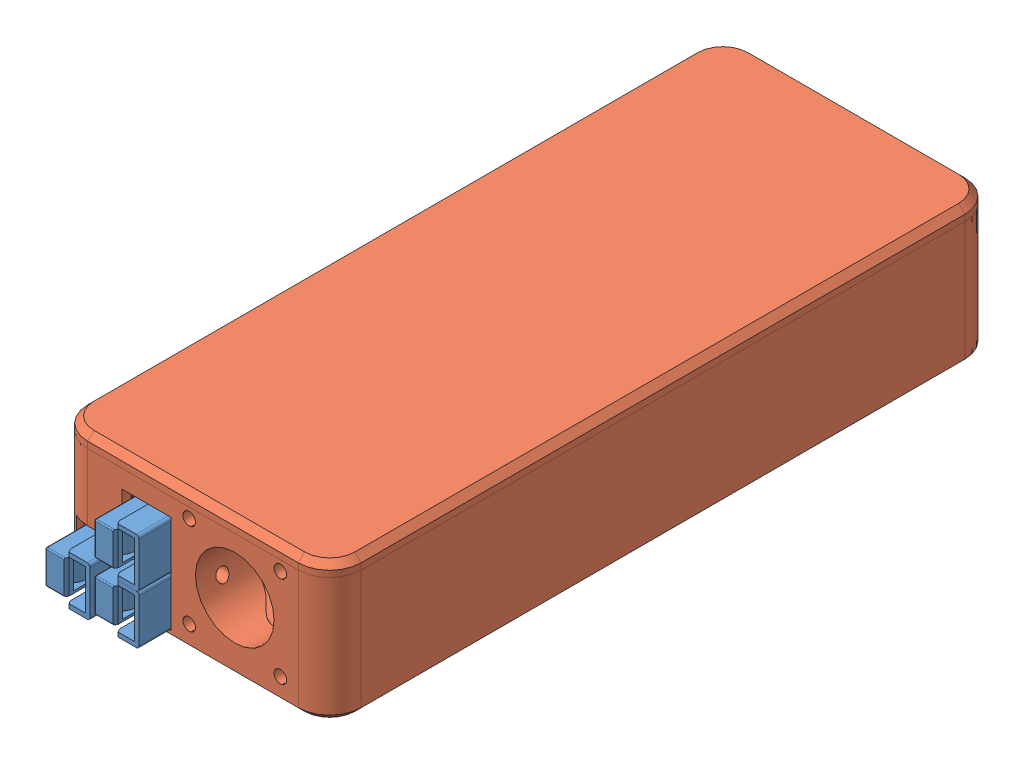
SolidWorks assembly AxxSolder_Portable, configuration Default. Lengths in mm.
Overall size (43.5 41.05 111.1).
6 component instances, 3 part files, 9 mates.
Components (placement in the parent):
- Anderson_PowerPole-3: Anderson_PowerPole [Default] at (-7.3715 3.9141 34.4539) x (0 -1 0) z (0 0 1) size (16.24 16.24 22.71)
  - powerpole 15-45A housing.step-3: powerpole 15-45A housing.step [Default] at origin size (8.44 8.44 22.71)
  - powerpole 15-45A housing.step-5: powerpole 15-45A housing.step [Default] at (-7.8 0 0) size (8.44 8.44 22.71)
  - powerpole 15-45A housing.step-6: powerpole 15-45A housing.step [Default] at (0 -7.8 0) size (8.44 8.44 22.71)
- Encolsure_Portable-1: Encolsure_Portable [Default] at origin size (43.5 21.95 106)
- AxxSolder-2: AxxSolder [Default] at (19.48 8.25 -50.802) x (1 0 0) z (0 -1 0) size (39.06 82.5 39.41)
Mates (geometry in assembly coordinates):
- Coincident1: coincident aligned: plane of Encolsure_Portable-1 through (0 0 0) normal (0 0 1)
- Coincident2: coincident aligned: plane of Encolsure_Portable-1 through (0 0 0) normal (0 1 0)
- Coincident3: coincident aligned: plane of Encolsure_Portable-1 through (0 0 0) normal (1 0 0)
- Coincident4: coincident: plane of Encolsure_Portable-1 through (-15.24 8.25 29.2) normal (0 -1 0); plane of AxxSolder-2 through (-0.02 8.25 -9.552) normal (0 1 0)
- Concentric1: concentric: cylinder of Encolsure_Portable-1 through (-15.24 8.25 29.2) axis (0 1 0) radius 1; cylinder of AxxSolder-2 through (-15.24 8.26 29.2) axis (0 -1 0) radius 1.25
- Concentric2: concentric: cylinder of Encolsure_Portable-1 through (15.24 8.25 29.2) axis (0 1 0) radius 1; cylinder of AxxSolder-2 through (15.24 8.26 29.2) axis (0 -1 0) radius 1.25
- Coincident11: coincident anti-aligned: plane of Anderson_PowerPole-3/powerpole 15-45A housing.step-3 through (-3.45 7.8 58.1) normal (1 0 0); plane of Encolsure_Portable-1 through (-3.45 0 56.5) normal (-1 0 0)
- Coincident12: coincident anti-aligned: plane of Anderson_PowerPole-3/powerpole 15-45A housing.step-3 through (-3.45 0 58.1) normal (0 -1 0); plane of Encolsure_Portable-1 through (-16.75 0 48) normal (0 1 0)
- Distance1: distance = 5.1 mm aligned: plane of Anderson_PowerPole-3/powerpole 15-45A housing.step-3 through (-11.25 7.8 58.1) normal (0 0 1); plane of Encolsure_Portable-1 through (-16.75 -1.5 53) normal (0 0 1)
